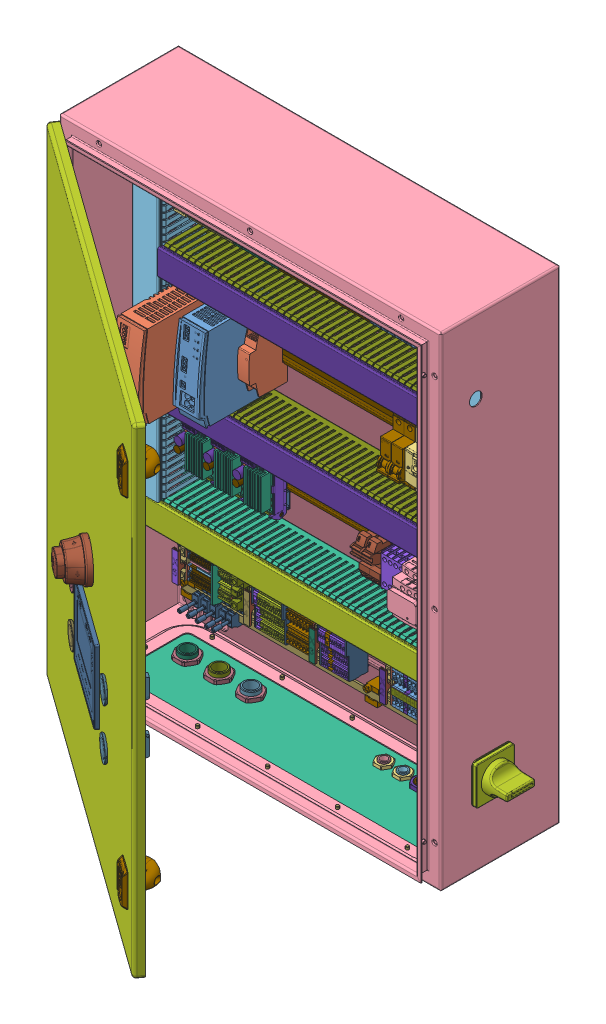
SolidWorks assembly Armoir életrique v46.step, configuration Valor predeterminado. Lengths in mm. (continued)
Components (placement in the parent): (continued)
- EM-241C_v4_2.step-1: EM-241C_v4_2.step [Valor predeterminado] at (-329.7091 5.608 81.2521) size (46 89.6 55.6) (continued)
  - DesignRootModel_2.step-1: DesignRootModel_2.step [Valor predeterminado] at origin size (42 72 25.9) (continued)
    - Submodel-CAP0603_100NF_part_simplified_0603_9.step-1: Submodel-CAP0603_100NF_part_simplified_0603_9.step [Valor predeterminado] at (432.9591 252.1852 -25.8521) x (0 -1 0) z (0 0 1) size (1.75 0.95 0.87) (continued)
      - Submodel-C_UsersTino Hellbergworks3D kokeilujaEM-241Cver4_PCB3DInput_SCAP 0603.xtd_33.step-1: Submodel-C_UsersTino Hellbergworks3D kokeilujaEM-241Cver4_PCB3DInput_SCAP 0603.xtd_33.step [Valor predeterminado] at (96.5835 -43.8059 11.5141) x (1 0 0) z (0 1 0) size (1.75 0.87 0.95)
        - CAP 0603.step-1: CAP 0603.step [Valor predeterminado] at origin size (1.75 0.87 0.95)
    - Submodel-CAP0603_100NF_part_simplified_0603_10.step-1: Submodel-CAP0603_100NF_part_simplified_0603_10.step [Valor predeterminado] at (431.4591 255.6852 -25.8521) x (0 -1 0) z (0 0 1) size (1.75 0.95 0.87)
      - Submodel-C_UsersTino Hellbergworks3D kokeilujaEM-241Cver4_PCB3DInput_SCAP 0603.xtd_34.step-1: Submodel-C_UsersTino Hellbergworks3D kokeilujaEM-241Cver4_PCB3DInput_SCAP 0603.xtd_34.step [Valor predeterminado] at (96.5835 -43.8059 11.5141) x (1 0 0) z (0 1 0) size (1.75 0.87 0.95)
        - CAP 0603.step-1: CAP 0603.step [Valor predeterminado] at origin size (1.75 0.87 0.95)
    - Submodel-CAP0603_100NF_part_simplified_0603_11.step-1: Submodel-CAP0603_100NF_part_simplified_0603_11.step [Valor predeterminado] at (419.4591 266.1852 -25.8521) size (1.75 0.95 0.87)
      - Submodel-C_UsersTino Hellbergworks3D kokeilujaEM-241Cver4_PCB3DInput_SCAP 0603.xtd_35.step-1: Submodel-C_UsersTino Hellbergworks3D kokeilujaEM-241Cver4_PCB3DInput_SCAP 0603.xtd_35.step [Valor predeterminado] at (96.5835 -43.8059 11.5141) x (1 0 0) z (0 1 0) size (1.75 0.87 0.95)
        - CAP 0603.step-1: CAP 0603.step [Valor predeterminado] at origin size (1.75 0.87 0.95)
    - Submodel-CAP0603_1NF_part_simplified_0603_16.step-1: Submodel-CAP0603_1NF_part_simplified_0603_16.step [Valor predeterminado] at (423.2091 277.1852 -25.8521) x (0 1 0) z (0 0 1) size (1.75 0.95 0.87)
      - Submodel-C_UsersTino Hellbergworks3D kokeilujaEM-241Cver4_PCB3DInput_SCAP 0603.xtd_36.step-1: Submodel-C_UsersTino Hellbergworks3D kokeilujaEM-241Cver4_PCB3DInput_SCAP 0603.xtd_36.step [Valor predeterminado] at (96.5835 -43.8059 11.5141) x (1 0 0) z (0 1 0) size (1.75 0.87 0.95)
        - CAP 0603.step-1: CAP 0603.step [Valor predeterminado] at origin size (1.75 0.87 0.95)
    - Submodel-CAP0603_1NF_part_simplified_0603_17.step-1: Submodel-CAP0603_1NF_part_simplified_0603_17.step [Valor predeterminado] at (423.9591 269.6852 -25.8521) x (0 1 0) z (0 0 1) size (1.75 0.95 0.87)
      - Submodel-C_UsersTino Hellbergworks3D kokeilujaEM-241Cver4_PCB3DInput_SCAP 0603.xtd_37.step-1: Submodel-C_UsersTino Hellbergworks3D kokeilujaEM-241Cver4_PCB3DInput_SCAP 0603.xtd_37.step [Valor predeterminado] at (96.5835 -43.8059 11.5141) x (1 0 0) z (0 1 0) size (1.75 0.87 0.95)
        - CAP 0603.step-1: CAP 0603.step [Valor predeterminado] at origin size (1.75 0.87 0.95)
    - Submodel-CAP0603_1NF_part_simplified_0603_18.step-1: Submodel-CAP0603_1NF_part_simplified_0603_18.step [Valor predeterminado] at (416.7091 265.4352 -25.8521) x (0 1 0) z (0 0 1) size (1.75 0.95 0.87)
      - Submodel-C_UsersTino Hellbergworks3D kokeilujaEM-241Cver4_PCB3DInput_SCAP 0603.xtd_38.step-1: Submodel-C_UsersTino Hellbergworks3D kokeilujaEM-241Cver4_PCB3DInput_SCAP 0603.xtd_38.step [Valor predeterminado] at (96.5835 -43.8059 11.5141) x (1 0 0) z (0 1 0) size (1.75 0.87 0.95)
        - CAP 0603.step-1: CAP 0603.step [Valor predeterminado] at origin size (1.75 0.87 0.95)
    - Submodel-CAP0603_1NF_part_simplified_0603_19.step-1: Submodel-CAP0603_1NF_part_simplified_0603_19.step [Valor predeterminado] at (416.7091 261.9352 -25.8521) x (0 1 0) z (0 0 1) size (1.75 0.95 0.87)
      - Submodel-C_UsersTino Hellbergworks3D kokeilujaEM-241Cver4_PCB3DInput_SCAP 0603.xtd_39.step-1: Submodel-C_UsersTino Hellbergworks3D kokeilujaEM-241Cver4_PCB3DInput_SCAP 0603.xtd_39.step [Valor predeterminado] at (96.5835 -43.8059 11.5141) x (1 0 0) z (0 1 0) size (1.75 0.87 0.95)
        - CAP 0603.step-1: CAP 0603.step [Valor predeterminado] at origin size (1.75 0.87 0.95)
    - Submodel-CAP0603_1NF_part_simplified_0603_20.step-1: Submodel-CAP0603_1NF_part_simplified_0603_20.step [Valor predeterminado] at (414.7091 261.9352 -25.8521) x (0 1 0) z (0 0 1) size (1.75 0.95 0.87)
      - Submodel-C_UsersTino Hellbergworks3D kokeilujaEM-241Cver4_PCB3DInput_SCAP 0603.xtd_40.step-1: Submodel-C_UsersTino Hellbergworks3D kokeilujaEM-241Cver4_PCB3DInput_SCAP 0603.xtd_40.step [Valor predeterminado] at (96.5835 -43.8059 11.5141) x (1 0 0) z (0 1 0) size (1.75 0.87 0.95)
        - CAP 0603.step-1: CAP 0603.step [Valor predeterminado] at origin size (1.75 0.87 0.95)
    - Submodel-CAP0603_1NF_part_simplified_0603_21.step-1: Submodel-CAP0603_1NF_part_simplified_0603_21.step [Valor predeterminado] at (414.7091 265.4352 -25.8521) x (0 -1 0) z (0 0 1) size (1.75 0.95 0.87)
      - Submodel-C_UsersTino Hellbergworks3D kokeilujaEM-241Cver4_PCB3DInput_SCAP 0603.xtd_41.step-1: Submodel-C_UsersTino Hellbergworks3D kokeilujaEM-241Cver4_PCB3DInput_SCAP 0603.xtd_41.step [Valor predeterminado] at (96.5835 -43.8059 11.5141) x (1 0 0) z (0 1 0) size (1.75 0.87 0.95)
        - CAP 0603.step-1: CAP 0603.step [Valor predeterminado] at origin size (1.75 0.87 0.95)
    - Submodel-CAP0603_1NF_part_simplified_0603_22.step-1: Submodel-CAP0603_1NF_part_simplified_0603_22.step [Valor predeterminado] at (425.2091 269.6852 -25.8521) x (0 1 0) z (0 0 1) size (1.75 0.95 0.87)
      - Submodel-C_UsersTino Hellbergworks3D kokeilujaEM-241Cver4_PCB3DInput_SCAP 0603.xtd_42.step-1: Submodel-C_UsersTino Hellbergworks3D kokeilujaEM-241Cver4_PCB3DInput_SCAP 0603.xtd_42.step [Valor predeterminado] at (96.5835 -43.8059 11.5141) x (1 0 0) z (0 1 0) size (1.75 0.87 0.95)
        - CAP 0603.step-1: CAP 0603.step [Valor predeterminado] at origin size (1.75 0.87 0.95)
    - Submodel-CAP0603_1NF_part_simplified_0603_23.step-1: Submodel-CAP0603_1NF_part_simplified_0603_23.step [Valor predeterminado] at (423.2091 284.6852 -25.8521) x (0 1 0) z (0 0 1) size (1.75 0.95 0.87)
      - Submodel-C_UsersTino Hellbergworks3D kokeilujaEM-241Cver4_PCB3DInput_SCAP 0603.xtd_43.step-1: Submodel-C_UsersTino Hellbergworks3D kokeilujaEM-241Cver4_PCB3DInput_SCAP 0603.xtd_43.step [Valor predeterminado] at (96.5835 -43.8059 11.5141) x (1 0 0) z (0 1 0) size (1.75 0.87 0.95)
        - CAP 0603.step-1: CAP 0603.step [Valor predeterminado] at origin size (1.75 0.87 0.95)
    - Submodel-CAP0603_2N2_part_simplified_0603_8.step-1: Submodel-CAP0603_2N2_part_simplified_0603_8.step [Valor predeterminado] at (423.2091 280.1852 -25.8521) x (0 1 0) z (0 0 1) size (1.75 0.95 0.87)
      - Submodel-C_UsersTino Hellbergworks3D kokeilujaEM-241Cver4_PCB3DInput_SCAP 0603.xtd_44.step-1: Submodel-C_UsersTino Hellbergworks3D kokeilujaEM-241Cver4_PCB3DInput_SCAP 0603.xtd_44.step [Valor predeterminado] at (96.5835 -43.8059 11.5141) x (1 0 0) z (0 1 0) size (1.75 0.87 0.95)
        - CAP 0603.step-1: CAP 0603.step [Valor predeterminado] at origin size (1.75 0.87 0.95)
    - Submodel-CAP0603_2N2_part_simplified_0603_9.step-1: Submodel-CAP0603_2N2_part_simplified_0603_9.step [Valor predeterminado] at (434.9591 285.6852 -25.8521) x (-1 0 0) z (0 0 1) size (1.75 0.95 0.87)
      - Submodel-C_UsersTino Hellbergworks3D kokeilujaEM-241Cver4_PCB3DInput_SCAP 0603.xtd_45.step-1: Submodel-C_UsersTino Hellbergworks3D kokeilujaEM-241Cver4_PCB3DInput_SCAP 0603.xtd_45.step [Valor predeterminado] at (96.5835 -43.8059 11.5141) x (1 0 0) z (0 1 0) size (1.75 0.87 0.95)
        - CAP 0603.step-1: CAP 0603.step [Valor predeterminado] at origin size (1.75 0.87 0.95)
    - Submodel-CAP0603_2N2_part_simplified_0603_10.step-1: Submodel-CAP0603_2N2_part_simplified_0603_10.step [Valor predeterminado] at (423.2091 287.6852 -25.8521) x (0 1 0) z (0 0 1) size (1.75 0.95 0.87)
      - Submodel-C_UsersTino Hellbergworks3D kokeilujaEM-241Cver4_PCB3DInput_SCAP 0603.xtd_46.step-1: Submodel-C_UsersTino Hellbergworks3D kokeilujaEM-241Cver4_PCB3DInput_SCAP 0603.xtd_46.step [Valor predeterminado] at (96.5835 -43.8059 11.5141) x (1 0 0) z (0 1 0) size (1.75 0.87 0.95)
        - CAP 0603.step-1: CAP 0603.step [Valor predeterminado] at origin size (1.75 0.87 0.95)
    - Submodel-CAP0603_2N2_part_simplified_0603_11.step-1: Submodel-CAP0603_2N2_part_simplified_0603_11.step [Valor predeterminado] at (434.7091 278.1852 -25.8521) x (-1 0 0) z (0 0 1) size (1.75 0.95 0.87)
      - Submodel-C_UsersTino Hellbergworks3D kokeilujaEM-241Cver4_PCB3DInput_SCAP 0603.xtd_47.step-1: Submodel-C_UsersTino Hellbergworks3D kokeilujaEM-241Cver4_PCB3DInput_SCAP 0603.xtd_47.step [Valor predeterminado] at (96.5835 -43.8059 11.5141) x (1 0 0) z (0 1 0) size (1.75 0.87 0.95)
        - CAP 0603.step-1: CAP 0603.step [Valor predeterminado] at origin size (1.75 0.87 0.95)
    - Submodel-7-215079-6_V_CON_MICROMATCH6_part_DIL6-V-2.54-MMATCH_2.step-1: Submodel-7-215079-6_V_CON_MICROMATCH6_part_DIL6-V-2.54-MMATCH_2.step [Valor predeterminado] at (399.7091 255.1852 -25.8521) x (0 1 0) z (0 0 1) size (9.56 5 7.15)
      - Submodel-C_UsersTino Hellbergworks3D kokeilujaEM-241Cver4_PCB3DImportedPartModelsc-7-215079-6-t-3d.step_2.step-1: Submodel-C_UsersTino Hellbergworks3D kokeilujaEM-241Cver4_PCB3DImportedPartModelsc-7-215079-6-t-3d.step_2.step [Valor predeterminado] at (0.0125 0 4.05) size (9.56 5 7.15)
        - c-7-215079-6-t-3d.step.step-1: c-7-215079-6-t-3d.step.step [Valor predeterminado] at origin size (9.56 5 7.15)
    - Submodel-PT1.5_slash_3-3.5-H_part_CON-H3-7.6_slash_9.2_slash_3.5_4.step-1: Submodel-PT1.5_slash_3-3.5-H_part_CON-H3-7.6_slash_9.2_slash_3.5_4.step [Valor predeterminado] at (407.4348 247.1852 -25.8521) size (11.2 7.55 13.65)
      - Submodel-C_UsersTino Hellbergworks3D kokeilujaEM-241Cver4_PCB3DImportedPartModelspxc_1984620_01_PT-1-5-3-3-5-H_3D.stp_4.step-1: Submodel-C_UsersTino Hellbergworks3D kokeilujaEM-241Cver4_PCB3DImportedPartModelspxc_1984620_01_PT-1-5-3-3-5-H_3D.stp_4.step [Valor predeterminado] at (-5.32 -3.925 0) size (11.2 7.55 13.65)
        - pxc_1984620_01_PT-1-5-3-3-5-H_3D.stp.step-1: pxc_1984620_01_PT-1-5-3-3-5-H_3D.stp.step [Valor predeterminado] at origin size (11.2 7.55 13.65)
    - Submodel-PT1.5_slash_2-3.5-H_part_CON-H2-7.6_slash_9.2_slash_3.5_4.step-1: Submodel-PT1.5_slash_2-3.5-H_part_CON-H2-7.6_slash_9.2_slash_3.5_4.step [Valor predeterminado] at (416.1852 247.1852 -25.8521) size (7.7 7.55 13.65)
      - Submodel-C_UsersTino Hellbergworks3D kokeilujaEM-241Cver4_PCB3DImportedPartModelspxc_1984617_01_PT-1-5-2-3-5-H_3D.stp_4.step-1: Submodel-C_UsersTino Hellbergworks3D kokeilujaEM-241Cver4_PCB3DImportedPartModelspxc_1984617_01_PT-1-5-2-3-5-H_3D.stp_4.step [Valor predeterminado] at (-3.52 -3.925 0) size (7.7 7.55 13.65)
        - pxc_1984617_01_PT-1-5-2-3-5-H_3D.stp.step-1: pxc_1984617_01_PT-1-5-2-3-5-H_3D.stp.step [Valor predeterminado] at origin size (7.7 7.55 13.65)
    - Submodel-PT1.5_slash_2-3.5-H_part_CON-H2-7.6_slash_9.2_slash_3.5_5.step-1: Submodel-PT1.5_slash_2-3.5-H_part_CON-H2-7.6_slash_9.2_slash_3.5_5.step [Valor predeterminado] at (423.1895 247.1852 -25.8521) size (7.7 7.55 13.65)
      - Submodel-C_UsersTino Hellbergworks3D kokeilujaEM-241Cver4_PCB3DImportedPartModelspxc_1984617_01_PT-1-5-2-3-5-H_3D.stp_5.step-1: Submodel-C_UsersTino Hellbergworks3D kokeilujaEM-241Cver4_PCB3DImportedPartModelspxc_1984617_01_PT-1-5-2-3-5-H_3D.stp_5.step [Valor predeterminado] at (-3.52 -3.925 0) size (7.7 7.55 13.65)
        - pxc_1984617_01_PT-1-5-2-3-5-H_3D.stp.step-1: pxc_1984617_01_PT-1-5-2-3-5-H_3D.stp.step [Valor predeterminado] at origin size (7.7 7.55 13.65)
    - Submodel-PT1.5_slash_3-3.5-H_part_CON-H3-7.6_slash_9.2_slash_3.5_5.step-1: Submodel-PT1.5_slash_3-3.5-H_part_CON-H3-7.6_slash_9.2_slash_3.5_5.step [Valor predeterminado] at (426.9591 305.1352 -25.8521) x (-1 0 0) z (0 0 1) size (11.2 7.55 13.65)
      - Submodel-C_UsersTino Hellbergworks3D kokeilujaEM-241Cver4_PCB3DImportedPartModelspxc_1984620_01_PT-1-5-3-3-5-H_3D.stp_5.step-1: Submodel-C_UsersTino Hellbergworks3D kokeilujaEM-241Cver4_PCB3DImportedPartModelspxc_1984620_01_PT-1-5-3-3-5-H_3D.stp_5.step [Valor predeterminado] at (-5.32 -3.925 0) size (11.2 7.55 13.65)
        - pxc_1984620_01_PT-1-5-3-3-5-H_3D.stp.step-1: pxc_1984620_01_PT-1-5-3-3-5-H_3D.stp.step [Valor predeterminado] at origin size (11.2 7.55 13.65)
    - Submodel-22-27-2071_V_MOLEX7-HEADER_2818368710_part_SIL7-V-2.54-MOLEX_NOSILK_2.step-1: Submodel-22-27-2071_V_MOLEX7-HEADER_2818368710_part_SIL7-V-2.54-MOLEX_NOSILK_2.step [Valor predeterminado] at (416.2091 244.3352 -25.8521) size (17.78 5.8 0.01)
      - Submodel-noModelForPart_22-27-2071_V_MOLEX7-HEADER_2818368710_2.step-1: Submodel-noModelForPart_22-27-2071_V_MOLEX7-HEADER_2818368710_2.step [Valor predeterminado] at origin size (17.78 5.8 0.01)
        - placementOutline.step-1: placementOutline.step [Valor predeterminado] at origin size (5.08 0.5 0.01)
        - placementOutline (1).step-1: placementOutline (1).step [Valor predeterminado] at origin size (5.08 1 0.01)
        - placementOutline (2).step-1: placementOutline (2).step [Valor predeterminado] at origin size (0.6 0.6 0.01)
        - placementOutline (3).step-1: placementOutline (3).step [Valor predeterminado] at origin size (0.3 0.3 0.01)
        - placementOutline (4).step-1: placementOutline (4).step [Valor predeterminado] at origin size (0.6 0.6 0.01)
        - placementOutline (5).step-1: placementOutline (5).step [Valor predeterminado] at origin size (0.3 0.3 0.01)
        - placementOutline (6).step-1: placementOutline (6).step [Valor predeterminado] at origin size (0.3 0.3 0.01)
        - placementOutline (7).step-1: placementOutline (7).step [Valor predeterminado] at origin size (0.6 0.6 0.01)
        - placementOutline (8).step-1: placementOutline (8).step [Valor predeterminado] at origin size (0.6 0.6 0.01)
        - placementOutline (9).step-1: placementOutline (9).step [Valor predeterminado] at origin size (0.3 0.3 0.01)
        - placementOutline (10).step-1: placementOutline (10).step [Valor predeterminado] at origin size (17.78 5.8 0.01)
        - placementOutline (11).step-1: placementOutline (11).step [Valor predeterminado] at origin size (5.08 0.5 0.01)
        - placementOutline (12).step-1: placementOutline (12).step [Valor predeterminado] at origin size (5.08 1 0.01)
        - placementOutline (13).step-1: placementOutline (13).step [Valor predeterminado] at origin size (0.6 0.6 0.01)
        - placementOutline (14).step-1: placementOutline (14).step [Valor predeterminado] at origin size (0.3 0.3 0.01)
        - placementOutline (15).step-1: placementOutline (15).step [Valor predeterminado] at origin size (0.6 0.6 0.01)
        - placementOutline (16).step-1: placementOutline (16).step [Valor predeterminado] at origin size (0.3 0.3 0.01)
        - placementOutline (17).step-1: placementOutline (17).step [Valor predeterminado] at origin size (0.3 0.3 0.01)
        - placementOutline (18).step-1: placementOutline (18).step [Valor predeterminado] at origin size (0.6 0.6 0.01)
    - Submodel-PT2.5_slash_2-5.0-H_part_CON-H2-9_slash_13.5_slash_5.0_4.step-1: Submodel-PT2.5_slash_2-5.0-H_part_CON-H2-9_slash_13.5_slash_5.0_4.step [Valor predeterminado] at (405.9723 305.9352 -25.8521) x (-1 0 0) z (0 0 1) size (10 9 17.6)
      - Submodel-C_UsersTino Hellbergworks3D kokeilujaEM-241Cver4_PCB3DImportedPartModelspxc_1935776_00_PT-2-5-2-5-0-H_3D.stp_4.step-1: Submodel-C_UsersTino Hellbergworks3D kokeilujaEM-241Cver4_PCB3DImportedPartModelspxc_1935776_00_PT-2-5-2-5-0-H_3D.stp_4.step [Valor predeterminado] at (13.9475 50.6993 -15.5526) x (0 -1 0) z (-1 0 0) size (9 17.6 10)
        - pxc_1935776_00_PT-2-5-2-5-0-H_3D.stp.step-1: pxc_1935776_00_PT-2-5-2-5-0-H_3D.stp.step [Valor predeterminado] at origin size (9 17.6 10)
    - Submodel-PT2.5_slash_2-5.0-H_part_CON-H2-9_slash_13.5_slash_5.0_5.step-1: Submodel-PT2.5_slash_2-5.0-H_part_CON-H2-9_slash_13.5_slash_5.0_5.step [Valor predeterminado] at (415.9527 305.9352 -25.8521) x (-1 0 0) z (0 0 1) size (10 9 17.6)
      - Submodel-C_UsersTino Hellbergworks3D kokeilujaEM-241Cver4_PCB3DImportedPartModelspxc_1935776_00_PT-2-5-2-5-0-H_3D.stp_5.step-1: Submodel-C_UsersTino Hellbergworks3D kokeilujaEM-241Cver4_PCB3DImportedPartModelspxc_1935776_00_PT-2-5-2-5-0-H_3D.stp_5.step [Valor predeterminado] at (13.9475 50.6993 -15.5526) x (0 -1 0) z (-1 0 0) size (9 17.6 10)
        - pxc_1935776_00_PT-2-5-2-5-0-H_3D.stp.step-1: pxc_1935776_00_PT-2-5-2-5-0-H_3D.stp.step [Valor predeterminado] at origin size (9 17.6 10)
    - Submodel-22-27-2031_V_MOLEX3-HEADER_3592429379_part_SIL3-V-2.54-MOLEX_NOSILK_2.step-1: Submodel-22-27-2031_V_MOLEX3-HEADER_3592429379_part_SIL3-V-2.54-MOLEX_NOSILK_2.step [Valor predeterminado] at (426.9591 307.9352 -25.8521) x (-1 0 0) z (0 0 1) size (7.6 5.8 0.01)
      - Submodel-noModelForPart_22-27-2031_V_MOLEX3-HEADER_3592429379_2.step-1: Submodel-noModelForPart_22-27-2031_V_MOLEX3-HEADER_3592429379_2.step [Valor predeterminado] at origin size (7.6 5.8 0.01)
        - placementOutline (19).step-1: placementOutline (19).step [Valor predeterminado] at origin size (7.6 5.8 0.01)
        - placementOutline (20).step-1: placementOutline (20).step [Valor predeterminado] at origin size (5.1 0.5 0.01)
        - placementOutline (21).step-1: placementOutline (21).step [Valor predeterminado] at origin size (5.1 1 0.01)
        - placementOutline (22).step-1: placementOutline (22).step [Valor predeterminado] at origin size (0.6 0.6 0.01)
        - placementOutline (23).step-1: placementOutline (23).step [Valor predeterminado] at origin size (0.3 0.3 0.01)
        - placementOutline (24).step-1: placementOutline (24).step [Valor predeterminado] at origin size (0.6 0.6 0.01)
        - placementOutline (25).step-1: placementOutline (25).step [Valor predeterminado] at origin size (0.3 0.3 0.01)
        - placementOutline (26).step-1: placementOutline (26).step [Valor predeterminado] at origin size (0.3 0.3 0.01)
        - placementOutline (27).step-1: placementOutline (27).step [Valor predeterminado] at origin size (0.6 0.6 0.01)
    - Submodel-SIL-SOCKET_2_RIBBON-2.54_part_SIL2-V-2.54_2.step-1: Submodel-SIL-SOCKET_2_RIBBON-2.54_part_SIL2-V-2.54_2.step [Valor predeterminado] at (428.4491 245.1252 -25.8521) x (0 1 0) z (0 0 1) size (5.08 2.54 7.37)
      - Submodel-C_UsersTino Hellbergworks3D kokeilujaEM-241Cver4_PCB3DImportedPartModelssil socket 2-way.STEP_2.step-1: Submodel-C_UsersTino Hellbergworks3D kokeilujaEM-241Cver4_PCB3DImportedPartModelssil socket 2-way.STEP_2.step [Valor predeterminado] at (-2.615 0.9644 4.266) x (0 -1 0) z (-1 0 0) size (2.54 7.37 5.08)
        - sil socket 2-way.STEP.step-1: sil socket 2-way.STEP.step [Valor predeterminado] at origin size (2.54 7.37 5.08)
    - Submodel-VDR_RAD_30VAC38VDC2J_1196060662_part_VDR-RAD-7.6_slash_2.6_slash_5.1_2.step-1: Submodel-VDR_RAD_30VAC38VDC2J_1196060662_part_VDR-RAD-7.6_slash_2.6_slash_5.1_2.step [Valor predeterminado] at (398.7091 297.9352 -25.8521) x (0 -1 0) z (0 0 1) size (7.28 3.6 7)
      - Submodel-noModelForPart_VDR_RAD_30VAC38VDC2J_1196060662_2.step-1: Submodel-noModelForPart_VDR_RAD_30VAC38VDC2J_1196060662_2.step [Valor predeterminado] at origin size (7.28 3.6 7)
        - placementOutline (28).step-1: placementOutline (28).step [Valor predeterminado] at origin size (7.28 3.6 7)
    - Submodel-NHDS-4_SMD-6.3_slash_6.7_slash_1.5_DIP4_part_SW-DIP4-6.3_slash_6.7_slash_1.5_2.step-1: Submodel-NHDS-4_SMD-6.3_slash_6.7_slash_1.5_DIP4_part_SW-DIP4-6.3_slash_6.7_slash_1.5_2.step [Valor predeterminado] at (400.4591 263.4352 -25.8521) x (0 -1 0) z (0 0 1) size (6.31 6.7 1.59)
      - Submodel-C_UsersTino Hellbergworks3D kokeilujaEM-241Cver4_PCB3DImportedPartModelsMCDHN-04.step_2.step-1: Submodel-C_UsersTino Hellbergworks3D kokeilujaEM-241Cver4_PCB3DImportedPartModelsMCDHN-04.step_2.step [Valor predeterminado] at (0.04 0.05 0.075) size (6.31 6.7 1.59)
        - MCDHN-04.step.step-1: MCDHN-04.step.step [Valor predeterminado] at origin size (6.31 6.7 1.59)
    - Submodel-RES1206_47R_part_1206_2.step-1: Submodel-RES1206_47R_part_1206_2.step [Valor predeterminado] at (434.4591 303.6852 -25.8521) x (0 1 0) z (0 0 1) size (3.35 1.73 0.85)
      - Submodel-C_UsersTino Hellbergworks3D kokeilujaEM-241Cver4_PCB3DImportedPartModelsRES-1206.step_2.step-1: Submodel-C_UsersTino Hellbergworks3D kokeilujaEM-241Cver4_PCB3DImportedPartModelsRES-1206.step_2.step [Valor predeterminado] x (1 0 0) z (0 -1 0) size (3.35 0.85 1.73)
        - RES-1206.step.step-1: RES-1206.step.step [Valor predeterminado] at origin size (3.35 0.85 1.73)
    - Submodel-RES1206_4K7_1006503616_part_1206_4.step-1: Submodel-RES1206_4K7_1006503616_part_1206_4.step [Valor predeterminado] at (423.9591 257.9352 -27.4521) x (-1 0 0) z (0 0 -1) size (3.2 1.5 0.6)
      - Submodel-noModelForPart_RES1206_4K7_1006503616_4.step-1: Submodel-noModelForPart_RES1206_4K7_1006503616_4.step [Valor predeterminado] at origin size (3.2 1.5 0.6)
        - placementOutline (29).step-1: placementOutline (29).step [Valor predeterminado] at origin size (3.2 1.5 0.6)
    - Submodel-RES1206_4K7_1006503616_part_1206_5.step-1: Submodel-RES1206_4K7_1006503616_part_1206_5.step [Valor predeterminado] at (423.9591 255.9352 -27.4521) x (-1 0 0) z (0 0 -1) size (3.2 1.5 0.6)
      - Submodel-noModelForPart_RES1206_4K7_1006503616_5.step-1: Submodel-noModelForPart_RES1206_4K7_1006503616_5.step [Valor predeterminado] at origin size (3.2 1.5 0.6)
        - placementOutline (29).step-1: placementOutline (29).step [Valor predeterminado] at origin size (3.2 1.5 0.6)
    - Submodel-RES_4527_0.01R3W_part_4527_2.step-1: Submodel-RES_4527_0.01R3W_part_4527_2.step [Valor predeterminado] at (429.4591 298.1852 -25.8521) x (-1 0 0) z (0 0 1) size (12.07 7.11 4.49)
      - Submodel-C_UsersTino Hellbergworks3D kokeilujaEM-241Cver4_PCB3DImportedPartModelsRES 4527.step_2.step-1: Submodel-C_UsersTino Hellbergworks3D kokeilujaEM-241Cver4_PCB3DImportedPartModelsRES 4527.step_2.step [Valor predeterminado] at (0 0 3.2591) x (1 0 0) z (0 -1 0) size (12.07 4.49 7.11)
        - RES 4527.step.step-1: RES 4527.step.step [Valor predeterminado] at origin size (12.07 4.49 7.11)
    - Submodel-MCP6001_SOT23-5_LOW_POWER_OPAMP_part_SOT23-5_2.step-1: Submodel-MCP6001_SOT23-5_LOW_POWER_OPAMP_part_SOT23-5_2.step [Valor predeterminado] at (433.9591 255.9352 -25.8521) x (-1 0 0) z (0 0 1) size (3 2.5 1.1)
      - Submodel-C_UsersTino Hellbergworks3D kokeilujaEM-241Cver4_PCB3DImportedPartModelsOT-23-5.step_2.step-1: Submodel-C_UsersTino Hellbergworks3D kokeilujaEM-241Cver4_PCB3DImportedPartModelsOT-23-5.step_2.step [Valor predeterminado] at (0 0 0.55) x (1 0 0) z (0 -1 0) size (3 1.1 2.5)
        - SOT-23-5.step.step-1: SOT-23-5.step.step [Valor predeterminado] at origin size (3 1.1 2.5)
    - Submodel-LM2936Z-5.0_TO92_715062582_part_TO92A_2.step-1: Submodel-LM2936Z-5.0_TO92_715062582_part_TO92A_2.step [Valor predeterminado] at (407.7091 274.4352 -25.8521) x (0 -1 0) z (0 0 1) size (3.54 2 0.01)
      - Submodel-noModelForPart_LM2936Z-5.0_TO92_715062582_2.step-1: Submodel-noModelForPart_LM2936Z-5.0_TO92_715062582_2.step [Valor predeterminado] at origin size (3.54 2 0.01)
        - placementOutline (30).step-1: placementOutline (30).step [Valor predeterminado] at origin size (3.54 2 0.01)
    - Submodel-CAPE_RAD_1000UF-35V-105C_12.9-21-5.1_1506459042_part_EL-RAD-12.9_slash_25.6_slash_5.1_2.step-1: Submodel-CAPE_RAD_1000UF-35V-105C_12.9-21-5.1_1506459042_part_EL-RAD-12.9_slash_25.6_slash_5.1_2.step [Valor predeterminado] at (402.385 287.7995 -25.8521) size (12.9 12.9 21)
      - Submodel-noModelForPart_CAPE_RAD_1000UF-35V-105C_12.9-21-5.1_1506459042_2.step-1: Submodel-noModelForPart_CAPE_RAD_1000UF-35V-105C_12.9-21-5.1_1506459042_2.step [Valor predeterminado] at origin size (12.9 12.9 21)
        - placementOutline (31).step-1: placementOutline (31).step [Valor predeterminado] at origin size (12.9 12.9 21)
    - Submodel-CAPE_RAD_470UF-35V-105C_10-20-5_3088446675_part_EL-RAD-10.5_slash_15.8_slash_5.1_2.step-1: Submodel-CAPE_RAD_470UF-35V-105C_10-20-5_3088446675_part_EL-RAD-10.5_slash_15.8_slash_5.1_2.step [Valor predeterminado] at (401.2091 275.9352 -25.8521) size (10.5 10.5 21.4)
      - Submodel-noModelForPart_CAPE_RAD_470UF-35V-105C_10-20-5_3088446675_2.step-1: Submodel-noModelForPart_CAPE_RAD_470UF-35V-105C_10-20-5_3088446675_2.step [Valor predeterminado] at origin size (10.5 10.5 21.4)
        - placementOutline (32).step-1: placementOutline (32).step [Valor predeterminado] at origin size (10.5 10.5 21.4)
    - Submodel-CAP0603_10NF_part_0603_4.step-1: Submodel-CAP0603_10NF_part_0603_4.step [Valor predeterminado] at (429.9591 252.1852 -25.8521) x (0 1 0) z (0 0 1) size (1.75 0.87 0.95)
      - Submodel-C_UsersTino Hellbergworks3D kokeilujaEM-241Cver4_PCB3DImportedPartModelsCAP 0603.stp_12.step-1: Submodel-C_UsersTino Hellbergworks3D kokeilujaEM-241Cver4_PCB3DImportedPartModelsCAP 0603.stp_12.step [Valor predeterminado] at (96.5835 -11.0791 -43.3309) size (1.75 0.87 0.95)
        - CAP 0603.stp.step-1: CAP 0603.stp.step [Valor predeterminado] at origin size (1.75 0.87 0.95)
    - Submodel-CAP0603_10NF_part_0603_5.step-1: Submodel-CAP0603_10NF_part_0603_5.step [Valor predeterminado] at (401.9591 268.6852 -25.8521) x (0 -1 0) z (0 0 1) size (1.75 0.87 0.95)
      - Submodel-C_UsersTino Hellbergworks3D kokeilujaEM-241Cver4_PCB3DImportedPartModelsCAP 0603.stp_13.step-1: Submodel-C_UsersTino Hellbergworks3D kokeilujaEM-241Cver4_PCB3DImportedPartModelsCAP 0603.stp_13.step [Valor predeterminado] at (96.5835 -11.0791 -43.3309) size (1.75 0.87 0.95)
        - CAP 0603.stp.step-1: CAP 0603.stp.step [Valor predeterminado] at origin size (1.75 0.87 0.95)
    - Submodel-CAP_RAD_1UF-63V_7-4.9-10.5-5_3810361828_part_CAP-RAD-7_slash_4.9_slash_10.5_slash_5_2.step-1: Submodel-CAP_RAD_1UF-63V_7-4.9-10.5-5_3810361828_part_CAP-RAD-7_slash_4.9_slash_10.5_slash_5_2.step [Valor predeterminado] at (404.9291 297.4352 -25.8521) size (7 4.9 9.5)
      - Submodel-noModelForPart_CAP_RAD_1UF-63V_7-4.9-10.5-5_3810361828_2.step-1: Submodel-noModelForPart_CAP_RAD_1UF-63V_7-4.9-10.5-5_3810361828_2.step [Valor predeterminado] at origin size (7 4.9 9.5)
        - placementOutline (33).step-1: placementOutline (33).step [Valor predeterminado] at origin size (7 4.9 9.5)
    - Submodel-CAPE_RAD_100UF-16V-105C_7-11-2.5_2855059144_part_EL-RAD-7_slash_11_slash_2.5_2.step-1: Submodel-CAPE_RAD_100UF-16V-105C_7-11-2.5_2855059144_part_EL-RAD-7_slash_11_slash_2.5_2.step [Valor predeterminado] at (406.2091 268.6852 -25.8521) size (7 7 11)
      - Submodel-noModelForPart_CAPE_RAD_100UF-16V-105C_7-11-2.5_2855059144_2.step-1: Submodel-noModelForPart_CAPE_RAD_100UF-16V-105C_7-11-2.5_2855059144_2.step [Valor predeterminado] at origin size (7 7 11)
        - placementOutline (34).step-1: placementOutline (34).step [Valor predeterminado] at origin size (7 7 11)
    - Submodel-CAP0603_47NF_part_0603_8.step-1: Submodel-CAP0603_47NF_part_0603_8.step [Valor predeterminado] at (404.4591 255.1852 -25.8521) size (1.75 0.87 0.95)
      - Submodel-C_UsersTino Hellbergworks3D kokeilujaEM-241Cver4_PCB3DImportedPartModelsCAP 0603.stp_14.step-1: Submodel-C_UsersTino Hellbergworks3D kokeilujaEM-241Cver4_PCB3DImportedPartModelsCAP 0603.stp_14.step [Valor predeterminado] at (96.5835 -11.0791 -43.3309) size (1.75 0.87 0.95)
        - CAP 0603.stp.step-1: CAP 0603.stp.step [Valor predeterminado] at origin size (1.75 0.87 0.95)
    - Submodel-CAP0603_47NF_part_0603_9.step-1: Submodel-CAP0603_47NF_part_0603_9.step [Valor predeterminado] at (409.9591 255.1852 -25.8521) size (1.75 0.87 0.95)
      - Submodel-C_UsersTino Hellbergworks3D kokeilujaEM-241Cver4_PCB3DImportedPartModelsCAP 0603.stp_15.step-1: Submodel-C_UsersTino Hellbergworks3D kokeilujaEM-241Cver4_PCB3DImportedPartModelsCAP 0603.stp_15.step [Valor predeterminado] at (96.5835 -11.0791 -43.3309) size (1.75 0.87 0.95)
        - CAP 0603.stp.step-1: CAP 0603.stp.step [Valor predeterminado] at origin size (1.75 0.87 0.95)
    - Submodel-CAP0603_47NF_part_0603_10.step-1: Submodel-CAP0603_47NF_part_0603_10.step [Valor predeterminado] at (413.9591 256.6852 -25.8521) x (0 -1 0) z (0 0 1) size (1.75 0.87 0.95)
      - Submodel-C_UsersTino Hellbergworks3D kokeilujaEM-241Cver4_PCB3DImportedPartModelsCAP 0603.stp_16.step-1: Submodel-C_UsersTino Hellbergworks3D kokeilujaEM-241Cver4_PCB3DImportedPartModelsCAP 0603.stp_16.step [Valor predeterminado] at (96.5835 -11.0791 -43.3309) size (1.75 0.87 0.95)
        - CAP 0603.stp.step-1: CAP 0603.stp.step [Valor predeterminado] at origin size (1.75 0.87 0.95)
    - Submodel-CAP0603_47NF_part_0603_11.step-1: Submodel-CAP0603_47NF_part_0603_11.step [Valor predeterminado] at (416.2091 257.1852 -25.8521) x (-1 0 0) z (0 0 1) size (1.75 0.87 0.95)
      - Submodel-C_UsersTino Hellbergworks3D kokeilujaEM-241Cver4_PCB3DImportedPartModelsCAP 0603.stp_17.step-1: Submodel-C_UsersTino Hellbergworks3D kokeilujaEM-241Cver4_PCB3DImportedPartModelsCAP 0603.stp_17.step [Valor predeterminado] at (96.5835 -11.0791 -43.3309) size (1.75 0.87 0.95)
        - CAP 0603.stp.step-1: CAP 0603.stp.step [Valor predeterminado] at origin size (1.75 0.87 0.95)
    - Submodel-LM317LM_SO8_part_SO8_2.step-1: Submodel-LM317LM_SO8_part_SO8_2.step [Valor predeterminado] at (412.4591 271.4352 -25.8521) size (4.9 5.78 1.45)
      - Submodel-C_UsersTino Hellbergworks3D kokeilujaEM-241Cver4_PCB3DImportedPartModelsO-8.step_2.step-1: Submodel-C_UsersTino Hellbergworks3D kokeilujaEM-241Cver4_PCB3DImportedPartModelsO-8.step_2.step [Valor predeterminado] at (-1.8923 -2.6289 0) x (0 1 0) z (1 0 0) size (5.78 1.45 4.9)
        - SO-8.step.step-1: SO-8.step.step [Valor predeterminado] at origin size (5.78 1.45 4.9)
    - Submodel-IRLR3705Z_DPAK_NMOS-55V-0.008R-LOGICLEV_part_DPAK_8.step-1: Submodel-IRLR3705Z_DPAK_NMOS-55V-0.008R-LOGICLEV_part_DPAK_8.step [Valor predeterminado] at (427.7091 278.9352 -25.8521) x (0 1 0) z (0 0 1) size (6.54 9.94 2.42)
      - Submodel-C_UsersTino Hellbergworks3D kokeilujaEM-241Cver4_PCB3DImportedPartModelsDPAK TO-252.step_8.step-1: Submodel-C_UsersTino Hellbergworks3D kokeilujaEM-241Cver4_PCB3DImportedPartModelsDPAK TO-252.step_8.step [Valor predeterminado] at (0 -1.4833 1.2725) x (1 0 0) z (0 -1 0) size (6.54 2.42 9.94)
        - DPAK TO-252.step.step-1: DPAK TO-252.step.step [Valor predeterminado] at origin size (6.54 2.42 9.94)
    - Submodel-IRLR3705Z_DPAK_NMOS-55V-0.008R-LOGICLEV_part_DPAK_9.step-1: Submodel-IRLR3705Z_DPAK_NMOS-55V-0.008R-LOGICLEV_part_DPAK_9.step [Valor predeterminado] at (413.7091 278.9352 -25.8521) x (0 1 0) z (0 0 1) size (6.54 9.94 2.42)
      - Submodel-C_UsersTino Hellbergworks3D kokeilujaEM-241Cver4_PCB3DImportedPartModelsDPAK TO-252.step_9.step-1: Submodel-C_UsersTino Hellbergworks3D kokeilujaEM-241Cver4_PCB3DImportedPartModelsDPAK TO-252.step_9.step [Valor predeterminado] at (0 -1.4833 1.2725) x (1 0 0) z (0 -1 0) size (6.54 2.42 9.94)
        - DPAK TO-252.step.step-1: DPAK TO-252.step.step [Valor predeterminado] at origin size (6.54 2.42 9.94)
    - Submodel-IRLR3705Z_DPAK_NMOS-55V-0.008R-LOGICLEV_part_DPAK_10.step-1: Submodel-IRLR3705Z_DPAK_NMOS-55V-0.008R-LOGICLEV_part_DPAK_10.step [Valor predeterminado] at (427.7091 286.4352 -25.8521) x (0 1 0) z (0 0 1) size (6.54 9.94 2.42)
      - Submodel-C_UsersTino Hellbergworks3D kokeilujaEM-241Cver4_PCB3DImportedPartModelsDPAK TO-252.step_10.step-1: Submodel-C_UsersTino Hellbergworks3D kokeilujaEM-241Cver4_PCB3DImportedPartModelsDPAK TO-252.step_10.step [Valor predeterminado] at (0 -1.4833 1.2725) x (1 0 0) z (0 -1 0) size (6.54 2.42 9.94)
        - DPAK TO-252.step.step-1: DPAK TO-252.step.step [Valor predeterminado] at origin size (6.54 2.42 9.94)
    - Submodel-IRLR3705Z_DPAK_NMOS-55V-0.008R-LOGICLEV_part_DPAK_11.step-1: Submodel-IRLR3705Z_DPAK_NMOS-55V-0.008R-LOGICLEV_part_DPAK_11.step [Valor predeterminado] at (413.7091 286.4352 -25.8521) x (0 1 0) z (0 0 1) size (6.54 9.94 2.42)
      - Submodel-C_UsersTino Hellbergworks3D kokeilujaEM-241Cver4_PCB3DImportedPartModelsDPAK TO-252.step_11.step-1: Submodel-C_UsersTino Hellbergworks3D kokeilujaEM-241Cver4_PCB3DImportedPartModelsDPAK TO-252.step_11.step [Valor predeterminado] at (0 -1.4833 1.2725) x (1 0 0) z (0 -1 0) size (6.54 2.42 9.94)
        - DPAK TO-252.step.step-1: DPAK TO-252.step.step [Valor predeterminado] at origin size (6.54 2.42 9.94)
    - uid__9223372036854778010.step-1: uid__9223372036854778010.step [Valor predeterminado] at (437.7091 312.9352 -27.4521) x (-1 0 0) z (0 0 1) size (42 72 1.6)
  - EM-KP72-42_5_2.step-1: EM-KP72-42_5_2.step [Valor predeterminado] at (417.7091 276.3913 -45.2521) x (0 1 0) z (0 0 1) size (89.6 46 37.6)
    - pxc_2907583_00_UM-72-PROFIL-100CM_3D_2.step-1: pxc_2907583_00_UM-72-PROFIL-100CM_3D_2.step [Valor predeterminado] at (0 -67.75 -8.2) x (1 0 0) z (0 -1 0) size (86.8 21.5 40)
      - UM_72-PROFIL_H.Select__00275083.step-1: UM_72-PROFIL_H.Select__00275083.step [Valor predeterminado] at (0 -7.8 -89.5) size (86.8 21.5 40)
    - pxc_2959337_01_UM-72-SE_3D_4.step-1: pxc_2959337_01_UM-72-SE_3D_4.step [Valor predeterminado] at (0 23 -8.5) x (1 0 0) z (0 -1 0) size (89.6 22.8 16)
      - UM_72-SE_H.Select__00276902.step-1: UM_72-SE_H.Select__00276902.step [Valor predeterminado] at (30.8924 14.4135 13) size (89.6 22.8 5)
      - Schr.Lins._3x14-Z_01151118.step-1: Schr.Lins._3x14-Z_01151118.step [Valor predeterminado] at (43.2572 8 73.95) x (1 0 0) z (0 0 -1) size (5.15 5.15 16)
      - Schr.Lins._3x14-Z_01151118.step-2: Schr.Lins._3x14-Z_01151118.step [Valor predeterminado] at (-36.4428 8 73.95) x (1 0 0) z (0 0 -1) size (5.15 5.15 16)
    - pxc_2959337_01_UM-72-SE_3D_5.step-1: pxc_2959337_01_UM-72-SE_3D_5.step [Valor predeterminado] at (0 -23 -8.5) x (-1 0 0) z (0 1 0) size (89.6 22.8 16)
      - UM_72-SE_H.Select__00276902.step-1: UM_72-SE_H.Select__00276902.step [Valor predeterminado] at (30.8924 14.4135 13) size (89.6 22.8 5)
      - Schr.Lins._3x14-Z_01151118.step-1: Schr.Lins._3x14-Z_01151118.step [Valor predeterminado] at (43.2572 8 73.95) x (1 0 0) z (0 0 -1) size (5.15 5.15 16)
      - Schr.Lins._3x14-Z_01151118.step-2: Schr.Lins._3x14-Z_01151118.step [Valor predeterminado] at (-36.4428 8 73.95) x (1 0 0) z (0 0 -1) size (5.15 5.15 16)
    - 39295.step-1: 39295.step [Valor predeterminado] at (0 18 -8.5) x (1 0 0) z (0 -1 0) size (85 18.1 11)
    - 39295.step-2: 39295.step [Valor predeterminado] at (0 -8 -8.5) x (1 0 0) z (0 -1 0) size (85 18.1 11)
- 2320513.step-1: 2320513.step [Valor predeterminado] at origin size (18 90.01 60.95)
  - STEP_PS_1AC_50DC_2-select.step-1: STEP_PS_1AC_50DC_2-select.step [Valor predeterminado] at (211.92 450.6981 20.1639) x (0 1 0) z (-1 0 0) size (90.01 60.95 18)
- 2964270.step-1: 2964270.step [Valor predeterminado] at (-510 0 120) size (18.3 79.6 54.3)
  - DEK-LED-L_YE-select.step-1: DEK-LED-L_YE-select.step [Valor predeterminado] at (574 562.3014 -136.7864) x (0 1 0) z (1 0 0) size (79.6 54.3 6.1)
  - DEK-LED-L_YE-select.step-2: DEK-LED-L_YE-select.step [Valor predeterminado] at (586.2 562.3014 -136.7864) x (0 1 0) z (1 0 0) size (79.6 54.3 6.1)
  - DEK-LED-L_YE-select.step-3: DEK-LED-L_YE-select.step [Valor predeterminado] at (580.1 562.3014 -136.7864) x (0 1 0) z (1 0 0) size (79.6 54.3 6.1)
- 1076.000(1).step-1: 1076.000(1).step [Valor predeterminado] at (-975 0 0) size (603.26 763.7 553.64)
  - _1076.000(1)_P1.step-1: _1076.000(1)_P1.step [Valor predeterminado] at (1272 -3 105) size (600 760 205.1)
  - _1XXX_01_04(B,1)_P7.step-1: _1XXX_01_04(B,1)_P7.step [Valor predeterminado] at (992.5 694.5 194.75) x (0 0 1) z (-1 0 0) size (16.07 66 15.75)
  - _1XXX_01_04(T,1)_P7.step-1: _1XXX_01_04(T,1)_P7.step [Valor predeterminado] at (992.5 59.5 194.75) x (0 0 1) z (-1 0 0) size (16.07 66 15.75)
  - _1676X_01_01(1)_P2.step-1: _1676X_01_01(1)_P2.step [Valor predeterminado] at (1210.221 376.9 378.3257) x (-0.811697 0 -0.584079) z (-0.584079 0 0.811697) size (595 755 17.5)
  - _6321.050_P9 1.step-1: _6321.050_P9 1.step [Valor predeterminado] at (1009.902 44 201.672) x (-1 0 0) z (0 0 -1) size (20.95 29.54 13.98)
  - _1XXX_01_05(1)_P8.step-1: _1XXX_01_05(1)_P8.step [Valor predeterminado] at (1413.1452 658.05 524.3454) x (0.811697 0 0.584079) z (0 -1 0) size (55.65 49.52 55.1)
  - _1XXX_01_05(1)_P8.step-2: _1XXX_01_05(1)_P8.step [Valor predeterminado] at (1413.1452 98.05 524.3454) x (0.811697 0 0.584079) z (0 -1 0) size (55.65 49.52 55.1)
  - _0000-00186369(1).step-1: _0000-00186369(1).step [Valor predeterminado] at (994 694.5 194.75) x (0 0 -1) z (0 1 0) size (10 7.19 10)
  - _0000-00186369(1).step-2: _0000-00186369(1).step [Valor predeterminado] at (994 59.5 194.75) x (0 0 -1) z (0 1 0) size (10 7.19 10)
  - _1XX7_04_00_7(1)_P5.step-1: _1XX7_04_00_7(1)_P5.step [Valor predeterminado] at (1272 -3.5 93.5) size (534 1.5 149)
  - _0000-00082819_P2.step-1: _0000-00082819_P2.step [Valor predeterminado] at (1013 -2.25 93.5) x (1 0 0) z (0 0 -1) size (11.5 13.2 11.5)
  - _0000-00082819_P2.step-2: _0000-00082819_P2.step [Valor predeterminado] at (1531 -2.25 93.5) x (1 0 0) z (0 0 -1) size (11.5 13.2 11.5)
  - _0000-00082819_P2.step-3: _0000-00082819_P2.step [Valor predeterminado] at (1052 -2.25 27) x (1 0 0) z (0 0 -1) size (11.5 13.2 11.5)
  - _0000-00082819_P2.step-4: _0000-00082819_P2.step [Valor predeterminado] at (1162 -2.25 27) x (1 0 0) z (0 0 -1) size (11.5 13.2 11.5)
  - _0000-00082819_P2.step-5: _0000-00082819_P2.step [Valor predeterminado] at (1272 -2.25 27) x (1 0 0) z (0 0 -1) size (11.5 13.2 11.5)
  - _0000-00082819_P2.step-6: _0000-00082819_P2.step [Valor predeterminado] at (1382 -2.25 27) x (1 0 0) z (0 0 -1) size (11.5 13.2 11.5)
  - _0000-00082819_P2.step-7: _0000-00082819_P2.step [Valor predeterminado] at (1492 -2.25 27) x (1 0 0) z (0 0 -1) size (11.5 13.2 11.5)
  - _0000-00082819_P2.step-8: _0000-00082819_P2.step [Valor predeterminado] at (1052 -2.25 160) x (1 0 0) z (0 0 -1) size (11.5 13.2 11.5)
  - _0000-00082819_P2.step-9: _0000-00082819_P2.step [Valor predeterminado] at (1162 -2.25 160) x (1 0 0) z (0 0 -1) size (11.5 13.2 11.5)
  - _0000-00082819_P2.step-10: _0000-00082819_P2.step [Valor predeterminado] at (1272 -2.25 160) x (1 0 0) z (0 0 -1) size (11.5 13.2 11.5)
  - _0000-00082819_P2.step-11: _0000-00082819_P2.step [Valor predeterminado] at (1382 -2.25 160) x (1 0 0) z (0 0 -1) size (11.5 13.2 11.5)
  - _0000-00082819_P2.step-12: _0000-00082819_P2.step [Valor predeterminado] at (1492 -2.25 160) x (1 0 0) z (0 0 -1) size (11.5 13.2 11.5)
  - _1676X_02_00(1)_P6.step-1: _1676X_02_00(1)_P6.step [Valor predeterminado] at (1272 22 20) size (550 735 2.5)
  - _0000-00168553(1).step-1: _0000-00168553(1).step [Valor predeterminado] at (1555.5 -3 16.5) size (20 6.85 20)
  - _0000-00189079(1).step-1: _0000-00189079(1).step [Valor predeterminado] at (1552 17 -1.55) x (1 0 0) z (0 0 -1) size (15.5 15.5 6.5)
  - _0000-00189079(1).step-2: _0000-00189079(1).step [Valor predeterminado] at (992 17 -1.55) x (1 0 0) z (0 0 -1) size (15.5 15.5 6.5)
  - _0000-00189079(1).step-3: _0000-00189079(1).step [Valor predeterminado] at (1552 737 -1.55) x (1 0 0) z (0 0 -1) size (15.5 15.5 6.5)
  - _0000-00189079(1).step-4: _0000-00189079(1).step [Valor predeterminado] at (992 737 -1.55) x (1 0 0) z (0 0 -1) size (15.5 15.5 6.5)
